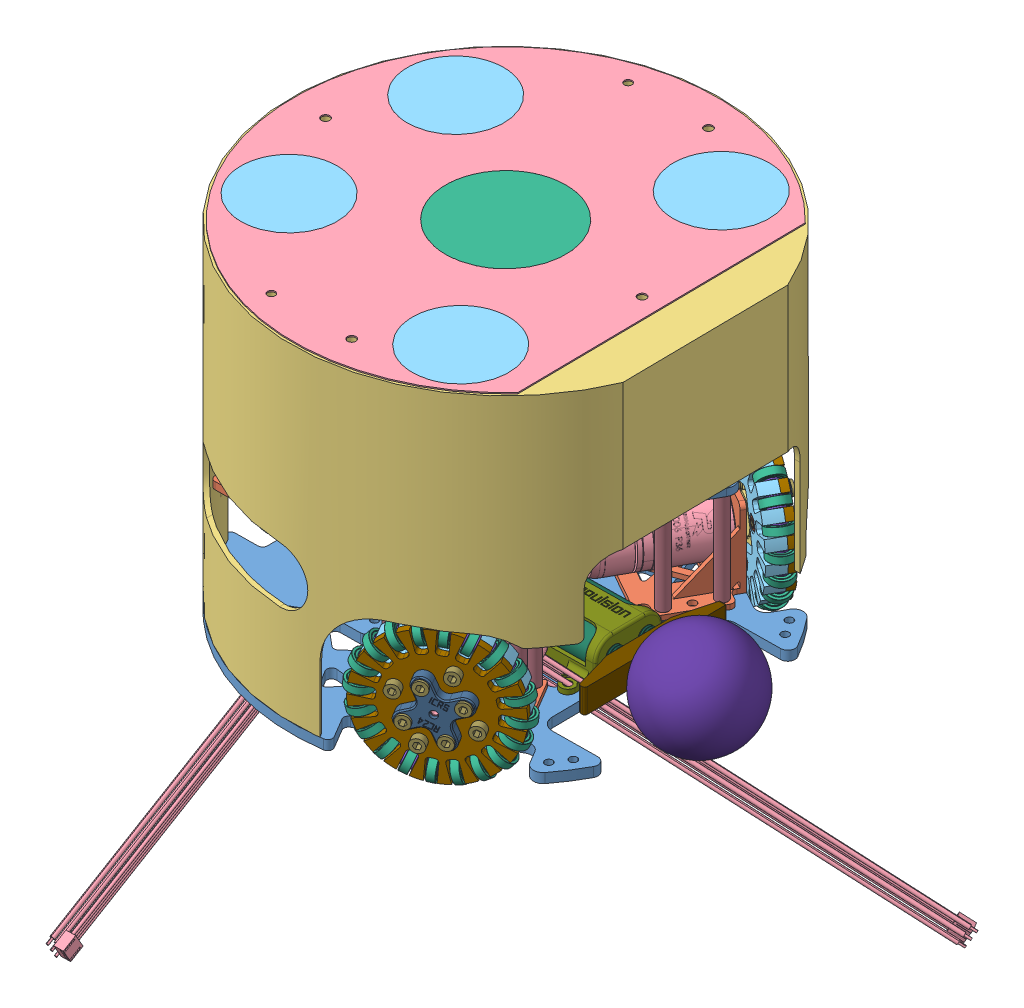
SolidWorks assembly ASM_ICRS_RCssl_2024_drive_base_Tri_wheel-intermediate, configuration Default. Lengths in mm. (continued)
Components (placement in the parent): (continued)
- RCSSL_gen2_OW_drive_unit-3: RCSSL_gen2_OW_drive_unit [Default] at (-93.2322 -22.9667 1.0926) x (-0.011698 0 -0.999932) z (0.999932 0 -0.011698) size (193.31 168.77 67.31)
  - 1.5mm_aluminium_metal_plating_2006 motor mount-1: 1.5mm_aluminium_metal_plating_2006 motor mount [Default] at (10.7348 39.9667 23.6101) size (46 32 35)
  - 3dp_AL_Gen2_Customised_AL_shaft_flange_connector_2006-1: 3dp_AL_Gen2_Customised_AL_shaft_flange_connector_2006 [Default] at (10.7348 39.9667 8.6101) x (0.866025 0.5 0) z (0 0 1) size (34 34 12.5)
  - RoboMaster M2006 P36 motor 1-1: RoboMaster M2006 P36 motor 1 [默认] at (29.0021 49.1921 55.5053) x (0.258819 0.965926 0) z (0 0 1) size (137.53 138.78 64.81)
  - ASM_RCssl_OW_Ver2-1: ASM_RCssl_OW_Ver2 [Default] at (25.0097 83.9716 -12.1645) x (-0.924615 -0.380903 0) z (0 0 1) size (59.33 59.33 15) (flexible)
    - 3dp_PETG_RCssl_OW_ver2_base-1: 3dp_PETG_RCssl_OW_ver2_base [Default] at (29.9603 35.2502 26.2746) size (54.84 54.84 7)
    - RCssl_OW_Ver2_roller_bearing_ASM-1: RCssl_OW_Ver2_roller_bearing_ASM [Default] at (24.4121 54.6156 21.3003) x (0 1 0) z (1 0 0) size (10 10 6)
      - BK_PU_68_3_10_3_bearing+roller-1: BK_PU_68_3_10_3_bearing+roller [Default] at (5.2981 6.4743 4.0482) size (10 10 3)
      - D3_H6_mid_axis-1: D3_H6_mid_axis [Default] at (5.2981 6.4743 2.5482) size (2.96 2.96 6)
      - m3_D6_H0.5_washer-1: m3_D6_H0.5_washer [Default] at (5.2981 6.4743 3.5482) x (0.872248 -0.489064 0) z (0 0 1) size (6 6 0.5)
      - m3_D6_H0.5_washer-2: m3_D6_H0.5_washer [Default] at (5.2981 6.4743 7.0482) size (6 6 0.5)
    - RCssl_OW_Ver2_roller_bearing_ASM-2: RCssl_OW_Ver2_roller_bearing_ASM [Default] at (30.6679 55.3823 21.3003) x (0.309017 0.951057 0) z (0.951057 -0.309017 0) size (10 10 6)
      - BK_PU_68_3_10_3_bearing+roller-1: BK_PU_68_3_10_3_bearing+roller [Default] at (5.2981 6.4743 4.0482) size (10 10 3)
      - D3_H6_mid_axis-1: D3_H6_mid_axis [Default] at (5.2981 6.4743 2.5482) size (2.96 2.96 6)
      - m3_D6_H0.5_washer-1: m3_D6_H0.5_washer [Default] at (5.2981 6.4743 3.5482) x (0.872248 -0.489064 0) z (0 0 1) size (6 6 0.5)
      - m3_D6_H0.5_washer-2: m3_D6_H0.5_washer [Default] at (5.2981 6.4743 7.0482) size (6 6 0.5)
    - RCssl_OW_Ver2_roller_bearing_ASM-3: RCssl_OW_Ver2_roller_bearing_ASM [Default] at (36.8544 54.1783 21.3003) x (0.587785 0.809017 0) z (0.809017 -0.587785 0) size (10 10 6)
      - BK_PU_68_3_10_3_bearing+roller-1: BK_PU_68_3_10_3_bearing+roller [Default] at (5.2981 6.4743 4.0482) size (10 10 3)
      - D3_H6_mid_axis-1: D3_H6_mid_axis [Default] at (5.2981 6.4743 2.5482) size (2.96 2.96 6)
      - m3_D6_H0.5_washer-1: m3_D6_H0.5_washer [Default] at (5.2981 6.4743 3.5482) x (0.872248 -0.489064 0) z (0 0 1) size (6 6 0.5)
      - m3_D6_H0.5_washer-2: m3_D6_H0.5_washer [Default] at (5.2981 6.4743 7.0482) size (6 6 0.5)
    - RCssl_OW_Ver2_roller_bearing_ASM-4: RCssl_OW_Ver2_roller_bearing_ASM [Default] at (42.3661 51.1215 21.3003) x (0.809017 0.587785 0) z (0.587785 -0.809017 0) size (10 10 6)
      - BK_PU_68_3_10_3_bearing+roller-1: BK_PU_68_3_10_3_bearing+roller [Default] at (5.2981 6.4743 4.0482) size (10 10 3)
      - D3_H6_mid_axis-1: D3_H6_mid_axis [Default] at (5.2981 6.4743 2.5482) size (2.96 2.96 6)
      - m3_D6_H0.5_washer-1: m3_D6_H0.5_washer [Default] at (5.2981 6.4743 3.5482) x (0.872248 -0.489064 0) z (0 0 1) size (6 6 0.5)
      - m3_D6_H0.5_washer-2: m3_D6_H0.5_washer [Default] at (5.2981 6.4743 7.0482) size (6 6 0.5)
    - RCssl_OW_Ver2_roller_bearing_ASM-5: RCssl_OW_Ver2_roller_bearing_ASM [Default] at (46.6634 46.5111 21.3003) x (0.951057 0.309017 0) z (0.309017 -0.951057 0) size (10 10 6)
      - BK_PU_68_3_10_3_bearing+roller-1: BK_PU_68_3_10_3_bearing+roller [Default] at (5.2981 6.4743 4.0482) size (10 10 3)
      - D3_H6_mid_axis-1: D3_H6_mid_axis [Default] at (5.2981 6.4743 2.5482) size (2.96 2.96 6)
      - m3_D6_H0.5_washer-1: m3_D6_H0.5_washer [Default] at (5.2981 6.4743 3.5482) x (0.872248 -0.489064 0) z (0 0 1) size (6 6 0.5)
      - m3_D6_H0.5_washer-2: m3_D6_H0.5_washer [Default] at (5.2981 6.4743 7.0482) size (6 6 0.5)
    - RCssl_OW_Ver2_roller_bearing_ASM-6: RCssl_OW_Ver2_roller_bearing_ASM [Default] at (49.3257 40.7985 21.3003) x (1 0 0) z (0 -1 0) size (10 10 6)
      - BK_PU_68_3_10_3_bearing+roller-1: BK_PU_68_3_10_3_bearing+roller [Default] at (5.2981 6.4743 4.0482) size (10 10 3)
      - D3_H6_mid_axis-1: D3_H6_mid_axis [Default] at (5.2981 6.4743 2.5482) size (2.96 2.96 6)
      - m3_D6_H0.5_washer-1: m3_D6_H0.5_washer [Default] at (5.2981 6.4743 3.5482) x (0.872248 -0.489064 0) z (0 0 1) size (6 6 0.5)
      - m3_D6_H0.5_washer-2: m3_D6_H0.5_washer [Default] at (5.2981 6.4743 7.0482) size (6 6 0.5)
    - RCssl_OW_Ver2_roller_bearing_ASM-7: RCssl_OW_Ver2_roller_bearing_ASM [Default] at (50.0924 34.5427 21.3003) x (0.951057 -0.309017 0) z (-0.309017 -0.951057 0) size (10 10 6)
      - BK_PU_68_3_10_3_bearing+roller-1: BK_PU_68_3_10_3_bearing+roller [Default] at (5.2981 6.4743 4.0482) size (10 10 3)
      - D3_H6_mid_axis-1: D3_H6_mid_axis [Default] at (5.2981 6.4743 2.5482) size (2.96 2.96 6)
      - m3_D6_H0.5_washer-1: m3_D6_H0.5_washer [Default] at (5.2981 6.4743 3.5482) x (0.872248 -0.489064 0) z (0 0 1) size (6 6 0.5)
      - m3_D6_H0.5_washer-2: m3_D6_H0.5_washer [Default] at (5.2981 6.4743 7.0482) size (6 6 0.5)
    - RCssl_OW_Ver2_roller_bearing_ASM-8: RCssl_OW_Ver2_roller_bearing_ASM [Default] at (48.8884 28.3562 21.3003) x (0.809017 -0.587785 0) z (-0.587785 -0.809017 0) size (10 10 6)
      - BK_PU_68_3_10_3_bearing+roller-1: BK_PU_68_3_10_3_bearing+roller [Default] at (5.2981 6.4743 4.0482) size (10 10 3)
      - D3_H6_mid_axis-1: D3_H6_mid_axis [Default] at (5.2981 6.4743 2.5482) size (2.96 2.96 6)
      - m3_D6_H0.5_washer-1: m3_D6_H0.5_washer [Default] at (5.2981 6.4743 3.5482) x (0.872248 -0.489064 0) z (0 0 1) size (6 6 0.5)
      - m3_D6_H0.5_washer-2: m3_D6_H0.5_washer [Default] at (5.2981 6.4743 7.0482) size (6 6 0.5)
    - RCssl_OW_Ver2_roller_bearing_ASM-9: RCssl_OW_Ver2_roller_bearing_ASM [Default] at (45.8316 22.8445 21.3003) x (0.587785 -0.809017 0) z (-0.809017 -0.587785 0) size (10 10 6)
      - BK_PU_68_3_10_3_bearing+roller-1: BK_PU_68_3_10_3_bearing+roller [Default] at (5.2981 6.4743 4.0482) size (10 10 3)
      - D3_H6_mid_axis-1: D3_H6_mid_axis [Default] at (5.2981 6.4743 2.5482) size (2.96 2.96 6)
      - m3_D6_H0.5_washer-1: m3_D6_H0.5_washer [Default] at (5.2981 6.4743 3.5482) x (0.872248 -0.489064 0) z (0 0 1) size (6 6 0.5)
      - m3_D6_H0.5_washer-2: m3_D6_H0.5_washer [Default] at (5.2981 6.4743 7.0482) size (6 6 0.5)
    - RCssl_OW_Ver2_roller_bearing_ASM-10: RCssl_OW_Ver2_roller_bearing_ASM [Default] at (41.2212 18.5472 21.3003) x (0.309017 -0.951057 0) z (-0.951057 -0.309017 0) size (10 10 6)
      - BK_PU_68_3_10_3_bearing+roller-1: BK_PU_68_3_10_3_bearing+roller [Default] at (5.2981 6.4743 4.0482) size (10 10 3)
      - D3_H6_mid_axis-1: D3_H6_mid_axis [Default] at (5.2981 6.4743 2.5482) size (2.96 2.96 6)
      - m3_D6_H0.5_washer-1: m3_D6_H0.5_washer [Default] at (5.2981 6.4743 3.5482) x (0.872248 -0.489064 0) z (0 0 1) size (6 6 0.5)
      - m3_D6_H0.5_washer-2: m3_D6_H0.5_washer [Default] at (5.2981 6.4743 7.0482) size (6 6 0.5)
    - RCssl_OW_Ver2_roller_bearing_ASM-11: RCssl_OW_Ver2_roller_bearing_ASM [Default] at (35.5086 15.8849 21.3003) x (0 -1 0) z (-1 0 0) size (10 10 6)
      - BK_PU_68_3_10_3_bearing+roller-1: BK_PU_68_3_10_3_bearing+roller [Default] at (5.2981 6.4743 4.0482) size (10 10 3)
      - D3_H6_mid_axis-1: D3_H6_mid_axis [Default] at (5.2981 6.4743 2.5482) size (2.96 2.96 6)
      - m3_D6_H0.5_washer-1: m3_D6_H0.5_washer [Default] at (5.2981 6.4743 3.5482) x (0.872248 -0.489064 0) z (0 0 1) size (6 6 0.5)
      - m3_D6_H0.5_washer-2: m3_D6_H0.5_washer [Default] at (5.2981 6.4743 7.0482) size (6 6 0.5)
    - RCssl_OW_Ver2_roller_bearing_ASM-12: RCssl_OW_Ver2_roller_bearing_ASM [Default] at (29.2528 15.1182 21.3003) x (-0.309017 -0.951057 0) z (-0.951057 0.309017 0) size (10 10 6)
      - BK_PU_68_3_10_3_bearing+roller-1: BK_PU_68_3_10_3_bearing+roller [Default] at (5.2981 6.4743 4.0482) size (10 10 3)
      - D3_H6_mid_axis-1: D3_H6_mid_axis [Default] at (5.2981 6.4743 2.5482) size (2.96 2.96 6)
      - m3_D6_H0.5_washer-1: m3_D6_H0.5_washer [Default] at (5.2981 6.4743 3.5482) x (0.872248 -0.489064 0) z (0 0 1) size (6 6 0.5)
      - m3_D6_H0.5_washer-2: m3_D6_H0.5_washer [Default] at (5.2981 6.4743 7.0482) size (6 6 0.5)
    - RCssl_OW_Ver2_roller_bearing_ASM-13: RCssl_OW_Ver2_roller_bearing_ASM [Default] at (23.0663 16.3222 21.3003) x (-0.587785 -0.809017 0) z (-0.809017 0.587785 0) size (10 10 6)
      - BK_PU_68_3_10_3_bearing+roller-1: BK_PU_68_3_10_3_bearing+roller [Default] at (5.2981 6.4743 4.0482) size (10 10 3)
      - D3_H6_mid_axis-1: D3_H6_mid_axis [Default] at (5.2981 6.4743 2.5482) size (2.96 2.96 6)
      - m3_D6_H0.5_washer-1: m3_D6_H0.5_washer [Default] at (5.2981 6.4743 3.5482) x (0.872248 -0.489064 0) z (0 0 1) size (6 6 0.5)
      - m3_D6_H0.5_washer-2: m3_D6_H0.5_washer [Default] at (5.2981 6.4743 7.0482) size (6 6 0.5)
    - RCssl_OW_Ver2_roller_bearing_ASM-14: RCssl_OW_Ver2_roller_bearing_ASM [Default] at (17.5546 19.379 21.3003) x (-0.809017 -0.587785 0) z (-0.587785 0.809017 0) size (10 10 6)
      - BK_PU_68_3_10_3_bearing+roller-1: BK_PU_68_3_10_3_bearing+roller [Default] at (5.2981 6.4743 4.0482) size (10 10 3)
      - D3_H6_mid_axis-1: D3_H6_mid_axis [Default] at (5.2981 6.4743 2.5482) size (2.96 2.96 6)
      - m3_D6_H0.5_washer-1: m3_D6_H0.5_washer [Default] at (5.2981 6.4743 3.5482) x (0.872248 -0.489064 0) z (0 0 1) size (6 6 0.5)
      - m3_D6_H0.5_washer-2: m3_D6_H0.5_washer [Default] at (5.2981 6.4743 7.0482) size (6 6 0.5)
    - RCssl_OW_Ver2_roller_bearing_ASM-15: RCssl_OW_Ver2_roller_bearing_ASM [Default] at (13.2573 23.9893 21.3003) x (-0.951057 -0.309017 0) z (-0.309017 0.951057 0) size (10 10 6)
      - BK_PU_68_3_10_3_bearing+roller-1: BK_PU_68_3_10_3_bearing+roller [Default] at (5.2981 6.4743 4.0482) size (10 10 3)
      - D3_H6_mid_axis-1: D3_H6_mid_axis [Default] at (5.2981 6.4743 2.5482) size (2.96 2.96 6)
      - m3_D6_H0.5_washer-1: m3_D6_H0.5_washer [Default] at (5.2981 6.4743 3.5482) x (0.872248 -0.489064 0) z (0 0 1) size (6 6 0.5)
      - m3_D6_H0.5_washer-2: m3_D6_H0.5_washer [Default] at (5.2981 6.4743 7.0482) size (6 6 0.5)
    - RCssl_OW_Ver2_roller_bearing_ASM-16: RCssl_OW_Ver2_roller_bearing_ASM [Default] at (10.595 29.702 21.3003) x (-1 0 0) z (0 1 0) size (10 10 6)
      - BK_PU_68_3_10_3_bearing+roller-1: BK_PU_68_3_10_3_bearing+roller [Default] at (5.2981 6.4743 4.0482) size (10 10 3)
      - D3_H6_mid_axis-1: D3_H6_mid_axis [Default] at (5.2981 6.4743 2.5482) size (2.96 2.96 6)
      - m3_D6_H0.5_washer-1: m3_D6_H0.5_washer [Default] at (5.2981 6.4743 3.5482) x (0.872248 -0.489064 0) z (0 0 1) size (6 6 0.5)
      - m3_D6_H0.5_washer-2: m3_D6_H0.5_washer [Default] at (5.2981 6.4743 7.0482) size (6 6 0.5)
    - RCssl_OW_Ver2_roller_bearing_ASM-17: RCssl_OW_Ver2_roller_bearing_ASM [Default] at (9.8283 35.9578 21.3003) x (-0.951057 0.309017 0) z (0.309017 0.951057 0) size (10 10 6)
      - BK_PU_68_3_10_3_bearing+roller-1: BK_PU_68_3_10_3_bearing+roller [Default] at (5.2981 6.4743 4.0482) size (10 10 3)
      - D3_H6_mid_axis-1: D3_H6_mid_axis [Default] at (5.2981 6.4743 2.5482) size (2.96 2.96 6)
      - m3_D6_H0.5_washer-1: m3_D6_H0.5_washer [Default] at (5.2981 6.4743 3.5482) x (0.872248 -0.489064 0) z (0 0 1) size (6 6 0.5)
      - m3_D6_H0.5_washer-2: m3_D6_H0.5_washer [Default] at (5.2981 6.4743 7.0482) size (6 6 0.5)
    - RCssl_OW_Ver2_roller_bearing_ASM-18: RCssl_OW_Ver2_roller_bearing_ASM [Default] at (11.0323 42.1443 21.3003) x (-0.809017 0.587785 0) z (0.587785 0.809017 0) size (10 10 6)
      - BK_PU_68_3_10_3_bearing+roller-1: BK_PU_68_3_10_3_bearing+roller [Default] at (5.2981 6.4743 4.0482) size (10 10 3)
      - D3_H6_mid_axis-1: D3_H6_mid_axis [Default] at (5.2981 6.4743 2.5482) size (2.96 2.96 6)
      - m3_D6_H0.5_washer-1: m3_D6_H0.5_washer [Default] at (5.2981 6.4743 3.5482) x (0.872248 -0.489064 0) z (0 0 1) size (6 6 0.5)
      - m3_D6_H0.5_washer-2: m3_D6_H0.5_washer [Default] at (5.2981 6.4743 7.0482) size (6 6 0.5)
    - RCssl_OW_Ver2_roller_bearing_ASM-19: RCssl_OW_Ver2_roller_bearing_ASM [Default] at (14.0891 47.656 21.3003) x (-0.587785 0.809017 0) z (0.809017 0.587785 0) size (10 10 6) (flexible)
      - BK_PU_68_3_10_3_bearing+roller-1: BK_PU_68_3_10_3_bearing+roller [Default] at (5.2981 6.4743 4.0482) size (10 10 3)
      - D3_H6_mid_axis-1: D3_H6_mid_axis [Default] at (5.2981 6.4743 2.5482) size (2.96 2.96 6)
      - m3_D6_H0.5_washer-1: m3_D6_H0.5_washer [Default] at (5.2981 6.4743 3.5482) x (0.872248 -0.489064 0) z (0 0 1) size (6 6 0.5)
      - m3_D6_H0.5_washer-2: m3_D6_H0.5_washer [Default] at (5.2981 6.4743 7.0482) size (6 6 0.5)
    - RCssl_OW_Ver2_roller_bearing_ASM-20: RCssl_OW_Ver2_roller_bearing_ASM [Default] at (18.6994 51.9533 21.3003) x (-0.309017 0.951057 0) z (0.951057 0.309017 0) size (10 10 6)
      - BK_PU_68_3_10_3_bearing+roller-1: BK_PU_68_3_10_3_bearing+roller [Default] at (5.2981 6.4743 4.0482) size (10 10 3)
      - D3_H6_mid_axis-1: D3_H6_mid_axis [Default] at (5.2981 6.4743 2.5482) size (2.96 2.96 6)
      - m3_D6_H0.5_washer-1: m3_D6_H0.5_washer [Default] at (5.2981 6.4743 3.5482) x (0.872248 -0.489064 0) z (0 0 1) size (6 6 0.5)
      - m3_D6_H0.5_washer-2: m3_D6_H0.5_washer [Default] at (5.2981 6.4743 7.0482) size (6 6 0.5)
    - CF3mm_OW_gen2_output_plane-1: CF3mm_OW_gen2_output_plane [Default] at (29.9603 35.2502 44.7746) size (54.84 54.84 3)
    - 3dp_PETG_RCssl_OW_front_lock-1: 3dp_PETG_RCssl_OW_front_lock [Default] at (29.9603 35.2502 21.2746) x (1 0 0) z (0 0 -1) size (21.15 21.15 4.13)
    - nut_din_985-m3x0_5-8-1: nut_din_985-m3x0_5-8 [Default] at (29.9603 21.2502 29.2746) x (-1 0 0) z (0 0 -1) size (6.2 5.5 4)
    - nut_din_985-m3x0_5-8-2: nut_din_985-m3x0_5-8 [Default] at (15.9603 35.2502 29.2746) x (0 1 0) z (0 0 -1) size (6.2 5.5 4)
    - nut_din_985-m3x0_5-8-3: nut_din_985-m3x0_5-8 [Default] at (29.9603 49.2502 29.2746) x (1 0 0) z (0 0 -1) size (6.2 5.5 4)
    - nut_din_985-m3x0_5-8-4: nut_din_985-m3x0_5-8 [Default] at (43.9603 35.2502 29.2746) x (0 -1 0) z (0 0 -1) size (6.2 5.5 4)
    - M3_304__full_teeth__screw_10mm-1: M3_304__full_teeth__screw_10mm [Default] at (29.992 49.2503 23.2746) x (-0.002323 0.999997 0) z (0 0 -1) size (5.3 5.3 13)
    - M3_304__full_teeth__screw_10mm-2: M3_304__full_teeth__screw_10mm [Default] at (43.9604 35.2186 23.2746) x (0.999997 0.002323 0) z (0 0 -1) size (5.3 5.3 13)
    - M3_304__full_teeth__screw_10mm-3: M3_304__full_teeth__screw_10mm [Default] at (29.9287 21.2502 23.2746) x (0.002323 -0.999997 0) z (0 0 -1) size (5.3 5.3 13)
    - M3_304__full_teeth__screw_10mm-4: M3_304__full_teeth__screw_10mm [Default] at (15.9603 35.2819 23.2746) x (-0.999997 -0.002323 0) z (0 0 -1) size (5.3 5.3 13)
    - M3_304__full_teeth__screw_10mm-5: M3_304__full_teeth__screw_10mm [Default] at (37.0442 42.2923 21.2746) x (0.914728 0.40407 0) z (0 0 -1) size (5.3 5.3 13)
    - M3_304__full_teeth__screw_10mm-6: M3_304__full_teeth__screw_10mm [Default] at (37.0024 28.1664 21.2746) x (0.40407 -0.914728 0) z (0 0 -1) size (5.3 5.3 13)
    - M3_304__full_teeth__screw_10mm-7: M3_304__full_teeth__screw_10mm [Default] at (22.8765 28.2081 21.2746) x (-0.914728 -0.40407 0) z (0 0 -1) size (5.3 5.3 13)
    - M3_304__full_teeth__screw_10mm-8: M3_304__full_teeth__screw_10mm [Default] at (22.9182 42.3341 21.2746) x (-0.40407 0.914728 0) z (0 0 -1) size (5.3 5.3 13)
  - AL_pillar_M3_D6_H40_Threaded-2: AL_pillar_M3_D6_H40_Threaded [H30] at (-8.7652 24.9667 50.1101) size (5 40 5)
  - AL_pillar_M3_D6_H40_Threaded-3: AL_pillar_M3_D6_H40_Threaded [H30] at (30.2348 24.9667 50.1101) size (5 40 5)
  - AL_pillar_M3_D6_H40_Threaded-4: AL_pillar_M3_D6_H40_Threaded [Default] at (30.2348 24.9667 32.1101) x (0.546545 0 0.83743) z (-0.83743 0 0.546545) size (5 40 5)
  - AL_pillar_M3_D6_H40_Threaded-5: AL_pillar_M3_D6_H40_Threaded [Default] at (-8.7652 24.9667 32.1101) x (0.546545 0 0.83743) z (-0.83743 0 0.546545) size (5 40 5)
- 24v0.85A_or_12v_0.428A_solenoid_10MM_travel_D12.7_H84-1: 24v0.85A_or_12v_0.428A_solenoid_10MM_travel_D12.7_H84 [Default] at (94.9244 17.6955 -52.5908) x (-0.014689 -0.08737 0.996068) z (-0.999892 0.002302 -0.014543) size (14.55 12.7 84.3)
  - Pin_24v0.85A_or_12v_0.428A_solenoid_10MM_travel_D12.7_H84-1: Pin_24v0.85A_or_12v_0.428A_solenoid_10MM_travel_D12.7_H84 [Default] at (36.4789 -6 68.9247) x (0.271091 0.962527 -0.007143) z (0.02634 0 0.999653) size (10 10 84)
  - Stator_24v0.85A_or_12v_0.428A_solenoid_10MM_travel_D12.7_H84-1: Stator_24v0.85A_or_12v_0.428A_solenoid_10MM_travel_D12.7_H84 [Default] at (36.5685 -6 72.3235) x (-0.999653 0 0.02634) z (-0.02634 0 -0.999653) size (12.7 12.7 58.2)
- 24v0.85A_or_12v_0.428A_solenoid_10MM_travel_D12.7_H84-2: 24v0.85A_or_12v_0.428A_solenoid_10MM_travel_D12.7_H84 [Default] at (95.0746 14.69 -39.7486) x (-0.014644 0 0.999893) z (-0.999893 0 -0.014644) size (14.55 12.7 84.3)
  - Pin_24v0.85A_or_12v_0.428A_solenoid_10MM_travel_D12.7_H84-1: Pin_24v0.85A_or_12v_0.428A_solenoid_10MM_travel_D12.7_H84 [Default] at (36.4789 -6 68.9247) x (0.271091 0.962527 -0.007143) z (0.02634 0 0.999653) size (10 10 84)
  - Stator_24v0.85A_or_12v_0.428A_solenoid_10MM_travel_D12.7_H84-1: Stator_24v0.85A_or_12v_0.428A_solenoid_10MM_travel_D12.7_H84 [Default] at (36.5685 -6 72.3235) x (-0.999653 0 0.02634) z (-0.02634 0 -0.999653) size (12.7 12.7 58.2)
- 3d_PETG_solenoid_holder-1: 3d_PETG_solenoid_holder [Default] at (5.9455 0 -10.8032) x (-0.011698 0 -0.999932) z (0.999932 0 -0.011698) size (179.88 19.4 163.58)
- 42mm_large_bullet-2: 42mm_large_bullet [Default] at (80.0937 8.685 -10.3031) x (-0.750349 0.660934 -0.011991) z (-0.432282 -0.476879 0.765322) size (42.7 42.7 42.7)
- 3DP_PETG_kicker_front_cap-1: 3DP_PETG_kicker_front_cap [Default] at (54.0422 3.69 -11.3659) x (0.999932 0 -0.011698) z (0.011698 0 0.999932) size (38.26 10 60)
- main_PCB_v1 - Copy-1: main_PCB_v1 - Copy [Default] at (-30.2368 45 -41.8737) x (0.011698 0 0.999932) z (0 1 0) size (107.15 95.52 20.5)
- CF3mm_battery_hub-1: CF3mm_battery_hub [Default] at (-61.0218 42 9.4815) x (0.999932 0 -0.011698) z (0.011698 0 0.999932) size (115.64 3 90.77)
- 3d_PETG_outer_shell - Copy-2: 3d_PETG_outer_shell - Copy [Default] at (4.6176 68 398.9672) x (0.999932 0 -0.011698) z (0 1 0) size (190.36 219.81 136)
- Upper_Cap-1: Upper_Cap [默认] at (-2.8104 -3.3591 73.8744) x (0.004362 0.008322 0.999956) z (-0.000065 0.999965 -0.008322) size (177.11 153.29 1.97)
  - colorcode-1: colorcode [默认] at (-83.4268 2.4294 140.0582) x (0.999938 0.007336 -0.008322) z (0.008322 0.000029 0.999965) size (176 152 0.5)
  - idcolor-1: idcolor [默认] at (-138.4525 37.0266 140.5151) x (-0.400562 -0.916263 0.00336) z (0.008322 0.000029 0.999965) size (40 40 0.5)
  - teamcolor-1: teamcolor [默认] at (-83.4268 2.4294 140.0582) x (0.999965 0 -0.008322) z (0.008322 0.000029 0.999965) size (50 50 0.5)
  - idcolor-2: idcolor [默认] at (-118.0228 -52.5982 140.3477) x (0.999965 0 -0.008322) z (0.008322 0.000029 0.999965) size (40 40 0.5)
  - idcolor-3: idcolor [默认] at (-48.0271 -52.0846 139.7651) x (0.999965 0 -0.008322) z (0.008322 0.000029 0.999965) size (40 40 0.5)
  - idcolor-4: idcolor [默认] at (-28.9147 37.8303 139.6035) x (0.999965 0 -0.008322) z (0.008322 0.000029 0.999965) size (40 40 0.5)
Mates (geometry in assembly coordinates):
- Concentric1: concentric anti-aligned: cylinder of CF4mm_RCssl_drive_base_ground_Tri_wheel-1 through (37.0644 0 -38.2252) axis (0 -1 0) radius 1.6; cylinder of RCSSL_gen2_OW_drive_unit-1/1.5mm_aluminium_metal_plating_2006 motor mount-1 through (37.0644 -25.9615 -38.2252) axis (0 1 0) radius 1.6
- Concentric2: concentric anti-aligned: cylinder of CF4mm_RCssl_drive_base_ground_Tri_wheel-1 through (45.8814 0 -53.9179) axis (0 -1 0) radius 1.6; cylinder of RCSSL_gen2_OW_drive_unit-1/1.5mm_aluminium_metal_plating_2006 motor mount-1 through (45.8814 -25.9615 -53.9179) axis (0 1 0) radius 1.6
- Coincident1: coincident anti-aligned: plane of CF4mm_RCssl_drive_base_ground_Tri_wheel-1 through (-0.754 0 -10.7249) normal (0 1 0); plane of RCSSL_gen2_OW_drive_unit-1/1.5mm_aluminium_metal_plating_2006 motor mount-1 through (15.9004 0 -40.3666) normal (0 -1 0)
- Concentric3: concentric anti-aligned: cylinder of CF4mm_RCssl_drive_base_ground_Tri_wheel-1 through (-43.4792 0 -29.7264) axis (0 -1 0) radius 1.6; cylinder of RCSSL_gen2_OW_drive_unit-3/1.5mm_aluminium_metal_plating_2006 motor mount-1 through (-43.4792 -25.9615 -29.7264) axis (0 1 0) radius 1.6
- Concentric4: concentric anti-aligned: cylinder of CF4mm_RCssl_drive_base_ground_Tri_wheel-1 through (-61.478 0 -29.5158) axis (0 -1 0) radius 1.6; cylinder of RCSSL_gen2_OW_drive_unit-3/1.5mm_aluminium_metal_plating_2006 motor mount-1 through (-61.478 -25.9615 -29.5158) axis (0 1 0) radius 1.6
- Coincident2: coincident anti-aligned: plane of CF4mm_RCssl_drive_base_ground_Tri_wheel-1 through (-0.754 0 -10.7249) normal (0 1 0); plane of RCSSL_gen2_OW_drive_unit-3/1.5mm_aluminium_metal_plating_2006 motor mount-1 through (-34.7517 0 -10.3271) normal (0 -1 0)
- Concentric5: concentric anti-aligned: cylinder of CF4mm_RCssl_drive_base_ground_Tri_wheel-1 through (4.1528 0 35.777) axis (0 -1 0) radius 1.6; cylinder of RCSSL_gen2_OW_drive_unit-2/1.5mm_aluminium_metal_plating_2006 motor mount-1 through (4.1528 -25.9615 35.777) axis (0 1 0) radius 1.6
- Concentric6: concentric anti-aligned: cylinder of CF4mm_RCssl_drive_base_ground_Tri_wheel-1 through (8.7437 0 43.5181) axis (0 -1 0) radius 1.6; cylinder of RCSSL_gen2_OW_drive_unit-2/1.5mm_aluminium_metal_plating_2006 motor mount-1 through (8.7437 -25.9615 43.5181) axis (0 1 0) radius 1.6
- Coincident3: coincident anti-aligned: plane of CF4mm_RCssl_drive_base_ground_Tri_wheel-1 through (-0.754 0 -10.7249) normal (0 1 0); plane of RCSSL_gen2_OW_drive_unit-2/1.5mm_aluminium_metal_plating_2006 motor mount-1 through (16.5893 0 18.5191) normal (0 -1 0)
- Coincident4: coincident aligned: plane of CF4mm_RCssl_drive_base_ground_Tri_wheel-1 through (-0.754 0 -10.7249) normal (0 1 0)
- Concentric7: concentric anti-aligned: cylinder of CF4mm_RCssl_drive_base_ground_Tri_wheel-1 through (46.8791 0 31.3654) axis (0 -1 0) radius 1.6; cylinder of RCSSL_gen2_OW_drive_unit-2/1.5mm_aluminium_metal_plating_2006 motor mount-1 through (46.8791 -25.9615 31.3654) axis (0 1 0) radius 1.6
- Parallel1: parallel aligned: plane of CF4mm_RCssl_drive_base_ground_Tri_wheel-1 through (51.3833 -10 27.115) normal (0.999932 0 -0.011698); plane of battery+ChargeMount_assembly-1/Battery-1 through (117.9683 72.75 -203.2458) normal (0.999932 0 -0.011698)
- Width1: width aligned: plane of battery+ChargeMount_assembly-1/RoboMaster 电池架-1 through (40.0943 50.95 -150.7312) normal (0.011698 0 0.999932); plane of battery+ChargeMount_assembly-1/RoboMaster 电池架-1 through (72.8642 72.7 -254.6217) normal (-0.011698 0 -0.999932); plane of CF4mm_RCssl_drive_base_ground_Tri_wheel-1 through (79.9574 -10 26.7807) normal (-0.011698 0 -0.999932); plane of CF4mm_RCssl_drive_base_ground_Tri_wheel-1 through (50.4838 -10 -49.7741) normal (0.011698 0 0.999932)
- Coincident9: coincident anti-aligned: plane of CF4mm_RCssl_drive_base_ground_Tri_wheel-1 through (-0.754 45 -10.7249) normal (0 1 0); plane of battery+ChargeMount_assembly-1/RoboMaster 电池架-1 through (59.3198 45 -258.3335) normal (0 -1 0)
- Coincident10: coincident aligned: plane of CF4mm_RCssl_drive_base_ground_Tri_wheel-1 through (51.3833 -10 27.115) normal (0.999932 0 -0.011698); plane of battery+ChargeMount_assembly-1/Battery-1 through (117.9683 72.75 -203.2458) normal (0.999932 0 -0.011698)
- Parallel2: parallel anti-aligned: plane of CF4mm_RCssl_drive_base_ground_Tri_wheel-1 through (-0.754 -4 -10.7249) normal (0 -1 0)
- Concentric18: concentric anti-aligned: cylinder of 24v0.85A_or_12v_0.428A_solenoid_10MM_travel_D12.7_H84-1/Stator_24v0.85A_or_12v_0.428A_solenoid_10MM_travel_D12.7_H84-1 through (22.0654 8.69 -17.7423) axis (0.999932 0 -0.011698) radius 6.35; cylinder of 3d_PETG_solenoid_holder-1 through (15.8659 8.69 -17.6697) axis (-0.999932 0 0.011698) radius 6.5
- Concentric19: concentric anti-aligned: cylinder of 24v0.85A_or_12v_0.428A_solenoid_10MM_travel_D12.7_H84-2/Stator_24v0.85A_or_12v_0.428A_solenoid_10MM_travel_D12.7_H84-1 through (22.2234 8.69 -4.2432) axis (0.999932 0 -0.011698) radius 6.35; cylinder of 3d_PETG_solenoid_holder-1 through (16.0238 8.69 -4.1707) axis (-0.999932 0 0.011698) radius 6.5
- Coincident16: coincident anti-aligned: plane of CF4mm_RCssl_drive_base_ground_Tri_wheel-1 through (-0.754 0 -10.7249) normal (0 1 0); plane of 3d_PETG_solenoid_holder-1 through (15.9448 0 -10.9202) normal (0 -1 0)
- Tangent1: tangent aligned: plane of CF4mm_RCssl_drive_base_ground_Tri_wheel-1 through (-0.754 -4 -10.7249) normal (0 -1 0); sphere of 42mm_large_bullet-1
- Concentric20: concentric anti-aligned: cylinder of CF4mm_RCssl_drive_base_ground_Tri_wheel-1 through (44.4769 -10 8.7474) axis (0 1 0) radius 1.6; cylinder of 3d_PETG_solenoid_holder-1 through (44.4769 3 8.7474) axis (0 -1 0) radius 1.6
- Concentric21: concentric anti-aligned: cylinder of CF4mm_RCssl_drive_base_ground_Tri_wheel-1 through (44.0089 -10 -31.2499) axis (0 1 0) radius 1.6; cylinder of 3d_PETG_solenoid_holder-1 through (44.0089 3 -31.2499) axis (0 -1 0) radius 1.6
- Coincident17: coincident anti-aligned: plane of 24v0.85A_or_12v_0.428A_solenoid_10MM_travel_D12.7_H84-2/Stator_24v0.85A_or_12v_0.428A_solenoid_10MM_travel_D12.7_H84-1 through (46.0217 8.69 -4.5216) normal (0.999932 0 -0.011698); plane of 3d_PETG_solenoid_holder-1 through (45.8638 8.69 -18.0207) normal (-0.999932 0 0.011698)
- Coincident18: coincident anti-aligned: plane of 24v0.85A_or_12v_0.428A_solenoid_10MM_travel_D12.7_H84-1/Stator_24v0.85A_or_12v_0.428A_solenoid_10MM_travel_D12.7_H84-1 through (45.8638 8.69 -18.0207) normal (0.999932 0 -0.011698); plane of 3d_PETG_solenoid_holder-1 through (45.8638 8.69 -18.0207) normal (-0.999932 0 0.011698)
- Parallel4: parallel aligned: plane of 24v0.85A_or_12v_0.428A_solenoid_10MM_travel_D12.7_H84-2/Stator_24v0.85A_or_12v_0.428A_solenoid_10MM_travel_D12.7_H84-1 through (22.2234 14.69 -4.2432) normal (0 1 0); plane of 3d_PETG_solenoid_holder-1 through (15.9448 16.19 -10.9202) normal (0 1 0)
- Tangent2: tangent anti-aligned: plane of CF4mm_RCssl_drive_base_ground_Tri_wheel-1 through (-0.754 -12.665 -10.7249) normal (0 1 0); sphere of 42mm_large_bullet-2
- Concentric23: concentric anti-aligned: cylinder of 24v0.85A_or_12v_0.428A_solenoid_10MM_travel_D12.7_H84-1/Pin_24v0.85A_or_12v_0.428A_solenoid_10MM_travel_D12.7_H84-1 through (53.9633 8.69 -18.1154) axis (0.999932 0 -0.011698) radius 1.25; cylinder of 3DP_PETG_kicker_front_cap-1 through (63.9626 8.69 -18.2324) axis (-0.999932 0 0.011698) radius 1.35
- Concentric24: concentric anti-aligned: cylinder of 24v0.85A_or_12v_0.428A_solenoid_10MM_travel_D12.7_H84-2/Pin_24v0.85A_or_12v_0.428A_solenoid_10MM_travel_D12.7_H84-1 through (54.1212 8.69 -4.6164) axis (0.999932 0 -0.011698) radius 1.25; cylinder of 3DP_PETG_kicker_front_cap-1 through (64.1205 8.69 -4.7333) axis (-0.999932 0 0.011698) radius 1.35
- Coincident20: coincident anti-aligned: plane of 24v0.85A_or_12v_0.428A_solenoid_10MM_travel_D12.7_H84-1/Stator_24v0.85A_or_12v_0.428A_solenoid_10MM_travel_D12.7_H84-1 through (53.9633 8.69 -18.1154) normal (0.999932 0 -0.011698); plane of 3DP_PETG_kicker_front_cap-1 through (54.0422 13.69 -11.3659) normal (-0.999932 0 0.011698)
- Concentric25: concentric: cylinder of CF4mm_RCssl_drive_base_ground_Tri_wheel-1 through (-0.754 0 -10.7249) axis (0 -1 0) radius 89; cylinder of 3d_PETG_outer_shell - Copy-1 through (-0.754 135.9879 -10.7249) axis (0 -1 0) radius 87
- Concentric28: concentric anti-aligned: cylinder of RCSSL_gen2_OW_drive_unit-1/AL_pillar_M3_D6_H40_Threaded-5 through (11.8806 42 -73.0215) axis (0 -1 0) radius 2.5; cylinder of main_PCB_v1 - Copy-1 through (11.8811 44.99 -73.0219) axis (0 1 0) radius 1.6
- Concentric29: concentric anti-aligned: cylinder of RCSSL_gen2_OW_drive_unit-3/AL_pillar_M3_D6_H40_Threaded-5 through (-61.0218 42 9.4815) axis (0 -1 0) radius 2.5; cylinder of main_PCB_v1 - Copy-1 through (-61.0218 44.99 9.4815) axis (0 1 0) radius 1.6
- Concentric30: concentric anti-aligned: cylinder of RCSSL_gen2_OW_drive_unit-3/AL_pillar_M3_D6_H40_Threaded-2 through (-43.023 42 9.271) axis (0 -1 0) radius 2.5; cylinder of main_PCB_v1 - Copy-1 through (-43.023 44.99 9.271) axis (0 1 0) radius 1.6
- Coincident22: coincident anti-aligned: plane of CF4mm_RCssl_drive_base_ground_Tri_wheel-1 through (-0.754 45 -10.7249) normal (0 1 0); plane of main_PCB_v1 - Copy-1 through (-33.9614 45 -40.4198) normal (0 -1 0)
- Coincident23: coincident anti-aligned: plane of CF4mm_RCssl_drive_base_ground_Tri_wheel-1 through (-0.754 0 -10.7249) normal (0 1 0); plane of 3d_PETG_outer_shell - Copy-1 through (-0.754 0 -10.7249) normal (0 -1 0)
- Concentric31: concentric aligned: cylinder of RCSSL_gen2_OW_drive_unit-2/AL_pillar_M3_D6_H40_Threaded-3 through (4.1528 42 35.777) axis (0 -1 0) radius 2.5; cylinder of CF3mm_battery_hub-1 through (4.1528 45 35.777) axis (0 -1 0) radius 1.6
- Concentric32: concentric anti-aligned: cylinder of RCSSL_gen2_OW_drive_unit-2/AL_pillar_M3_D6_H40_Threaded-2 through (37.6974 42 15.8832) axis (0 -1 0) radius 2.5; cylinder of CF3mm_battery_hub-1 through (37.6974 42 15.8832) axis (0 1 0) radius 4
- Coincident24: coincident anti-aligned: plane of RCSSL_gen2_OW_drive_unit-2/AL_pillar_M3_D6_H40_Threaded-2 through (37.6974 42 15.8832) normal (0 1 0); plane of CF3mm_battery_hub-1 through (-61.0218 42 9.4815) normal (0 -1 0)
- Concentric34: concentric aligned: cylinder of CF4mm_RCssl_drive_base_ground_Tri_wheel-1 through (-0.754 0 -10.7249) axis (0 -1 0) radius 89; cylinder of 3d_PETG_outer_shell - Copy-2 through (-0.754 136 -10.7249) axis (0 -1 0) radius 89
- Concentric36: concentric aligned: cylinder of CF4mm_RCssl_drive_base_ground_Tri_wheel-1 through (-14.7164 -12 71.0923) axis (0 1 0) radius 1.6; cylinder of 3d_PETG_outer_shell - Copy-2 through (-14.7164 -11.9879 71.0923) axis (0 1 0) radius 1.6
- Coincident25: coincident anti-aligned: plane of CF4mm_RCssl_drive_base_ground_Tri_wheel-1 through (-0.754 0 -10.7249) normal (0 1 0); plane of 3d_PETG_outer_shell - Copy-2 through (-0.754 0 -10.7249) normal (0 -1 0)
- Coincident26: coincident anti-aligned: plane of 3d_PETG_outer_shell - Copy-2 through (-0.754 136 -10.7249) normal (0 1 0); plane of Upper_Cap-1/colorcode-1 through (-0.754 136 -10.7249) normal (0 -1 0)
- Concentric42: concentric aligned: cylinder of 3d_PETG_outer_shell - Copy-2 through (-0.754 136 -10.7249) axis (0 -1 0) radius 89; cylinder of Upper_Cap-1/colorcode-1 through (-0.754 136.5 -10.7249) axis (0 -1 0) radius 88
- Parallel8: parallel aligned: plane of 3d_PETG_outer_shell - Copy-2 through (81.934 136 48.7773) normal (0.999932 0 -0.011698); plane of Upper_Cap-1/colorcode-1 through (62.5351 136.5 -71.8681) normal (0.999932 0 -0.011698)
